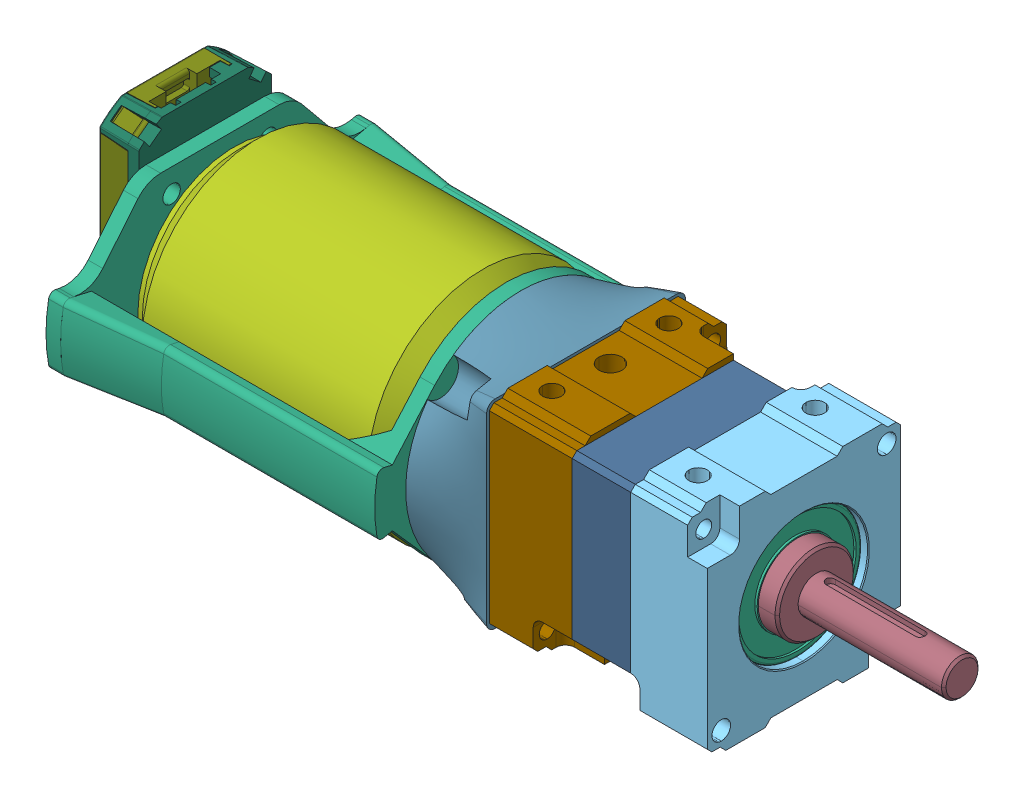
SolidWorks assembly PropDrive10to1, configuration Default. Lengths in mm.
Overall size (173.44 53.05 69.17).
46 component instances, 32 part files, 5 mates.
Components (placement in the parent):
- VersaPlanetary_v2_Single_Stage_10_1_with_BAG.STEP-1: VersaPlanetary_v2_Single_Stage_10_1_with_BAG.STEP [Default] at origin size (163.4 63.52 63.52)
  - 217-2820 Rev1_Public.STEP-1: 217-2820 Rev1_Public.STEP [Default] at (-4.6546 22.225 0) x (0 -0.456494 0.889726) z (-1 0 0) size (39.22 38.88 17.4)
    - 217-2625-100.STEP-1: 217-2625-100.STEP [Default] at origin size (39.22 38.88 12.7)
      - 217-2625-008 Rev1.STEP-1: 217-2625-008 Rev1.STEP [Default] at origin size (34.7 34.7 4.7)
      - 217-2625-010 Rev1.STEP-1: 217-2625-010 Rev1.STEP [Default] at (0 10.193 3.65) x (0.999813 0.019336 0) z (0 0 1) size (4 4 12)
      - 217-2625-010 Rev1.STEP-2: 217-2625-010 Rev1.STEP [Default] at (8.691 -5.3258 3.65) size (4 4 12)
      - 217-2625-010 Rev1.STEP-3: 217-2625-010 Rev1.STEP [Default] at (-8.691 -5.3258 3.65) size (4 4 12)
      - 217-2625-005 Rev1_Planet_Revolving_Follower01.STEP-1: 217-2625-005 Rev1_Planet_Revolving_Follower01.STEP [Default] at (8.691 -5.3258 6.35) x (0.932816 0.360354 0) z (0 0 1) size (16.89 16.89 8)
      - 217-2625-005 Rev1_Planet_Revolving_Follower01.STEP-2: 217-2625-005 Rev1_Planet_Revolving_Follower01.STEP [Default] at (-8.691 -5.3258 6.35) x (-0.932788 -0.360426 0) z (0 0 1) size (16.89 16.89 8)
      - 217-2625-005 Rev1_Planet_Revolving_Follower01.STEP-3: 217-2625-005 Rev1_Planet_Revolving_Follower01.STEP [Default] at (0 10.193 6.35) x (0.893583 0.448898 0) z (0 0 1) size (16.89 16.89 8)
    - 217-2625-007 Rev1_Public.STEP-1: 217-2625-007 Rev1_Public.STEP [Default] at (0 0 6.7) x (0.992772 0.120019 0) z (0 0 1) size (15.27 15.27 12.7)
  - 217-2625-026 Rev1.STEP-1: 217-2625-026 Rev1.STEP [Default] at (-6.5 22.225 0) x (0 -1 0) z (-1 0 0) size (44.45 42 18.12)
  - 217-2742-001 Rev4.STEP-1: 217-2742-001 Rev4.STEP [Default] at (0.2002 22.225 0) x (1 0 0) z (0 -0.092627 0.995701) size (7 28 28)
  - 217-2742-001 Rev4.STEP-2: 217-2742-001 Rev4.STEP [Default] at (8.2002 22.225 0) size (7 28 28)
  - 217-2625-017 Rev1_9714K61.STEP-1: 217-2625-017 Rev1_9714K61.STEP [Default] at (7.42 22.3002 -0.342) x (0 0.56703 0.823697) z (0 -0.823697 0.56703) size (28.51 4.98 27.43)
  - 217-2625-003 Rev1.STEP-1: 217-2625-003 Rev1.STEP [Default] at (7.4478 22.225 0) x (0 -1 0) z (1 0 0) size (17 17 64.11) (hidden)
  - 217-2625-018 Rev1_98541A410.STEP-1: 217-2625-018 Rev1_98541A410.STEP [Default] at (-0.7046 22.225 0) x (1 0 0) z (0 -0.017452 0.999848) size (1 19.6 17.4)
  - 832-1750-Ring-Gear-Screw_SSA0832-0500ZC.STEP-1: 832-1750-Ring-Gear-Screw_SSA0832-0500ZC.STEP [Default] at (-30.7 4.725 -17.5) x (0 0.997447 0.071411) z (0 -0.071411 0.997447) size (6.73 48.51 6.73) (hidden)
  - 832-1750-Ring-Gear-Screw_SSA0832-0500ZC.STEP-2: 832-1750-Ring-Gear-Screw_SSA0832-0500ZC.STEP [Default] at (-30.7 39.725 17.5) x (0 0.005929 0.999982) z (0 -0.999982 0.005929) size (6.73 48.51 6.73) (hidden)
  - 217-2625-025 Rev1.STEP-1: 217-2625-025 Rev1.STEP [Default] at (-23.2 22.225 0) x (0 -1 0) z (-1 0 0) size (44.45 42 18)
  - 217-4649-002 Rev1_SSA0832-0500ZC.STEP-1: 217-4649-002 Rev1_SSA0832-0500ZC.STEP [Default] at (-33.7 4.2645 17.9605) x (0 0.33842 -0.940995) z (0 0.940995 0.33842) size (6.73 16.76 6.73) (hidden)
  - 217-4649-002 Rev1_SSA0832-0500ZC.STEP-2: 217-4649-002 Rev1_SSA0832-0500ZC.STEP [Default] at (-33.7 40.1855 -17.9605) x (0 -0.308932 -0.951084) z (0 0.951084 -0.308932) size (6.73 16.76 6.73) (hidden)
  - 217-4649-006 Rev1_SSA0004-008BA.STEP-1: 217-4649-006 Rev1_SSA0004-008BA.STEP [Default] at (-30.7 22.225 12.5) x (0 0.5 -0.866025) z (0 -0.866025 -0.5) size (7 14 7) (hidden)
  - 217-4649-006 Rev1_SSA0004-008BA.STEP-2: 217-4649-006 Rev1_SSA0004-008BA.STEP [Default] at (-30.7 22.225 -12.5) x (0 -0.5 0.866025) z (0 0.866025 0.5) size (7 14 7) (hidden)
  - 217-2822-003 Rev4.STEP-1: 217-2822-003 Rev4.STEP [Default] at (-32.2 22.225 0) x (0 -1 0) z (-1 0 0) size (42 42 4.8) (hidden)
  - 217-3351 Rev2.STEP-1: 217-3351 Rev2.STEP [Default] at (-33.7 22.225 0) x (0 0 1) z (1 0 0) size (59.07 59.07 84.5) (hidden)
  - 217-2816-001 Rev1.STEP-1: 217-2816-001 Rev1.STEP [Default] at (-6.35 22.225 0) x (0 -1 0) z (1 0 0) size (42 42 14.51)
  - 217-4649-001 Rev1.STEP-1: 217-4649-001 Rev1.STEP [Default] at (-20.046 22.225 0) x (0 -1 0) z (1 0 0) size (18 18 13)
  - 217-4649-007 Rev1_94105A824.STEP-1: 217-4649-007 Rev1_94105A824.STEP [Default] at (-25.521 22.225 -6.7835) x (-0.996104 -0.088191 0) z (0 0 -1) size (4.83 4.83 4.77)
  - 217-2625-011 Rev1.STEP-1: 217-2625-011 Rev1.STEP [Default] at (-24.7818 22.225 0) x (0 0 1) z (0 -1 0) size (8.01 7.5 7.94) (hidden)
- VersaPlanetary_CIM_Motor_Output_Shaft_Kit_217-2893-1: VersaPlanetary_CIM_Motor_Output_Shaft_Kit_217-2893 [Default] at (7.4478 22.225 0) x (0 0 -1) z (1 0 0) size (17 17 57.85)
- PDAdapter^PropDrive10to1-1: PDAdapter^PropDrive10to1 [Default] at origin size (14.63 50.01 50.01) (virtual)
- 380kvMotorEncoded-1: 380kvMotorEncoded [Default] at (-48.0193 22.225 0) x (0 -1 0) z (0 0 -1) size (53.05 100.5 69.17)
  - CUI_DEVICES_AMT102-0048-N2000-S-1: CUI_DEVICES_AMT102-0048-N2000-S [Default] at (0 69.12 0) x (0 0 1) z (0 1 0) size (36.33 46.21 9.2)
    - CUI_DEVICES_AMT102-0048-N2000-S.step-1: CUI_DEVICES_AMT102-0048-N2000-S.step [Default] at origin size (36.33 46.21 9.2)
      - AMT-102-Base-REV-K.step-1: AMT-102-Base-REV-K.step [Default] x (-1 0 0) z (0 0 -1) size (28.78 43.39 9.06)
      - AMT-102-Top-Cover-REV-H.step-1: AMT-102-Top-Cover-REV-H.step [Default] at (0 0 5.23) x (-1 0 0) z (0 0 -1) size (28.6 43.26 6.55)
      - AMT-Sleeve-REV-D_ 2 mm.step-1: AMT-Sleeve-REV-D_ 2 mm.step [Default] at (0 0 -2.42) x (0.999996 0.002864 0) z (0 0 1) size (10.79 10.79 7.8)
      - AMT-Hub-Top-REV-D1.step-1: AMT-Hub-Top-REV-D1.step [Default] at (0 0 2.13) x (0.999996 0.002864 0) z (0 0 1) size (14 14 5.67)
      - AMT-Hub-Bottom-REV-B.step-1: AMT-Hub-Bottom-REV-B.step [Default] at (0 0 2.43) x (0.999998 -0.001942 0) z (0 0 1) size (17.3 17.3 3.2)
      - AMT10X-Shaft-Adaptor-REV-E.step-1: AMT10X-Shaft-Adaptor-REV-E.step [Default] at (0 0 0.03) x (0.999996 0.002864 0) z (0 0 1) size (11.8 11.8 7.8)
      - Receiver-board.step-1: Receiver-board.step [Default] at (72.2834 -20.351 3.03) x (-1 0 0) z (0 0 -1) size (26.5 26.62 0.41)
      - Rotor-board-REV F.step-1: Rotor-board-REV F.step [Default] at (0 0 2.13) x (0.807874 -0.589355 0) z (0 0 1) size (26 26 0.3)
      - Transmitter-board AMT10_AMT-102.step-1: Transmitter-board AMT10_AMT-102.step [Default] at (19.1596 -17.1102 1.22) x (-1 0 0) z (0 0 -1) size (26.63 38.43 4.41)
  - Body^380kvMotorEncoded-1: Body^380kvMotorEncoded [Default] at origin size (50 68.53 69.17) (virtual)
  - PROPDRIVE v2 5060 380KV Brushless Outrunner Motor-1: PROPDRIVE v2 5060 380KV Brushless Outrunner Motor [Default] x (1 0 0) z (0 0 -1) size (50 100 50)
Mates (geometry in assembly coordinates):
- Concentric2: concentric anti-aligned: cylinder of VersaPlanetary_v2_Single_Stage_10_1_with_BAG.STEP-1/217-2742-001 Rev4.STEP-2 through (8.2002 22.225 0) axis (-1 0 0) radius 7.5; cylinder of VersaPlanetary_CIM_Motor_Output_Shaft_Kit_217-2893-1 through (15.2002 22.225 0) axis (1 0 0) radius 8.5
- Coincident3: coincident anti-aligned: plane of VersaPlanetary_v2_Single_Stage_10_1_with_BAG.STEP-1/217-2742-001 Rev4.STEP-2 through (15.2002 29.725 0) normal (1 0 0); plane of VersaPlanetary_CIM_Motor_Output_Shaft_Kit_217-2893-1 through (15.2002 22.225 0) normal (-1 0 0)
- Concentric3: concentric aligned: cylinder of VersaPlanetary_v2_Single_Stage_10_1_with_BAG.STEP-1/217-4649-001 Rev1.STEP-1 through (-20.046 22.225 0) axis (-1 0 0) radius 4.005; cylinder of 380kvMotorEncoded-1/PROPDRIVE v2 5060 380KV Brushless Outrunner Motor-1 through (-22.0193 22.225 0) axis (-1 0 0) radius 2.5
- Parallel2: parallel anti-aligned: plane of 380kvMotorEncoded-1 through (-48.0193 22.225 0) normal (0 -1 0)
- Coincident7: coincident anti-aligned: plane of PDAdapter^PropDrive10to1-1 through (-44.8443 22.225 0) normal (-1 0 0); plane of 380kvMotorEncoded-1/Body^380kvMotorEncoded-1 through (-44.8443 22.225 0) normal (1 0 0)
